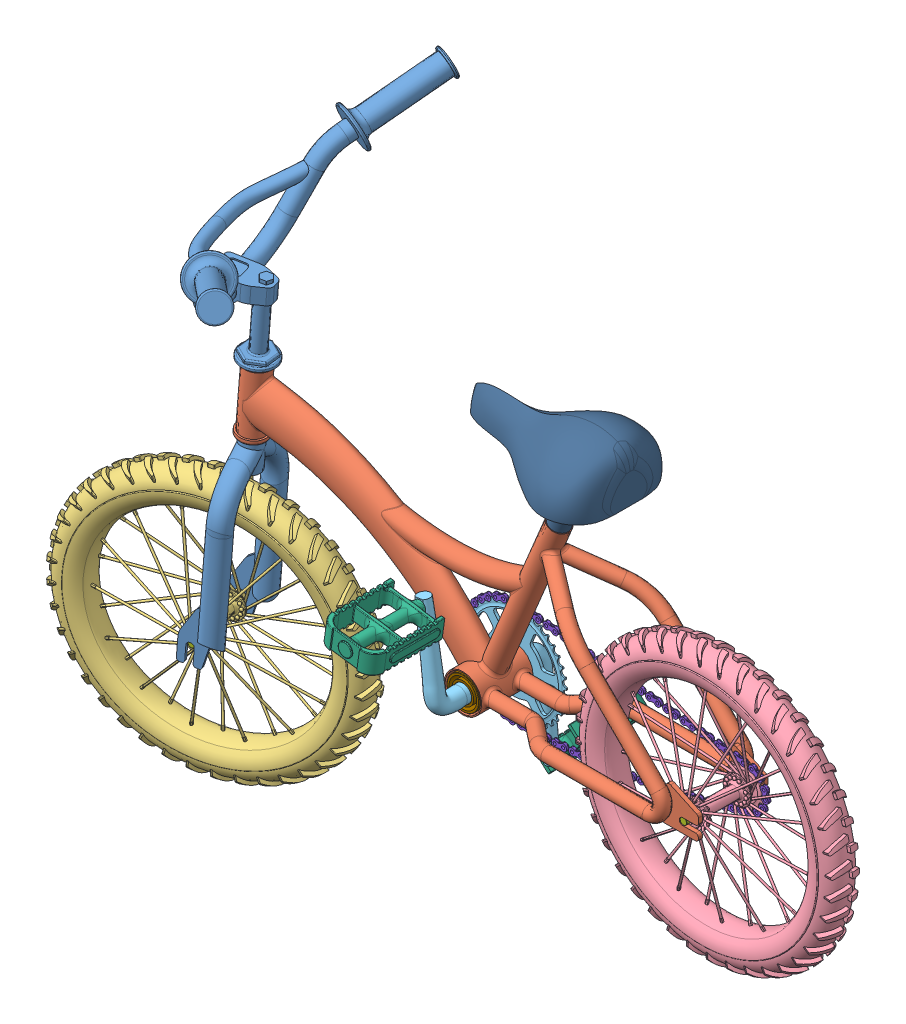
SolidWorks assembly Złożenierower, configuration Domyślna. Lengths in mm.
Overall size (1238.71 868.15 536.88).
12 component instances, 10 part files, 24 mates.
Components (placement in the parent):
- rower 1-1: rower 1 [Domyślna] at (-43.4947 150.1532 689.5871) x (0.960692 -0.078308 -0.266344) z (0.265464 -0.021639 0.963878) size (154.93 662.1 514.19)
- Część2-1: Część2 [Domyślna] at (307.1756 -163.303 684.2602) size (723.47 282.62 139.06)
- Część4-2: Część4 [Domyślna] at (-84.7109 -280.6724 691.2667) x (0.955551 -0.127096 -0.266024) z (0.265464 -0.021639 0.963878) size (399.15 399.28 100)
- Część3-1: Część3 [Domyślna] at (642.2913 -151.643 684.2602) x (0.731915 -0.681396 0) z (0 0 1) size (399.15 399.28 89)
- Część5-1: Część5 [Domyślna] at (307.1756 -163.303 685.2602) x (-0.14018 0.990126 0) z (0 0 1) size (270.08 150.67 176.37)
- Część9-1: Część9 [Domyślna] at (289.6531 -39.5372 827.2602) x (0 0 -1) z (0.990192 -0.139713 0) size (110.71 30.09 84)
- Część9-2: Część9 [Domyślna] at (324.6981 -287.0688 543.2602) x (0 0 1) z (0.66893 0.743326 0) size (110.71 30.09 84)
- Część8-1: Część8 [Domyślna] at (-84.7109 -280.6724 691.2667) x (0.911361 0.331819 -0.243551) z (0.265464 -0.021639 0.963878) size (10 10 100)
- Część8-2: Część8 [Domyślna] at (642.2913 -151.643 684.2602) x (1 -0.000733 0) z (0 0 1) size (10 10 100)
- Część7-2: Część7 [Domyślna] at (434.3029 -101.1447 643.7602) x (-0.994614 0.103648 0) z (0 0 -1) size (447.75 160.33 4)
- radial ball bearing_68_am-2: radial ball bearing_68_am [AFBMA 20.1 - 60-25 - 14,SI,NC,14_68] at (307.1756 -163.303 701.7602) x (0 0 -1) z (1 0 0) size (40 47 47)
- Część6-2: Część6 [Domyślna] at (397.1598 161.7409 684.2602) x (0.999017 -0.044322 0) z (0 0 1) size (231.81 225.72 159.65)
Mates (geometry in assembly coordinates):
- Koncentryczne1: concentric anti-aligned: cylinder of rower 1-1 through (-29.8866 79.8152 684.2602) axis (-0.081243 -0.996694 0) radius 15; cylinder of Część2-1 through (-51.9685 -191.087 684.2602) axis (0.081243 0.996694 0) radius 16
- Wspólnie2: coincident anti-aligned: plane of rower 1-1 through (-30.2928 74.8317 684.2602) normal (-0.081243 -0.996694 0); plane of Część2-1 through (-30.2928 74.8317 684.2602) normal (0.081243 0.996694 0)
- Koncentryczne3: concentric anti-aligned: cylinder of rower 1-1 through (-70.3758 -281.8409 743.3161) axis (-0.265464 0.021639 -0.963878) radius 5; cylinder of Część4-2 through (-94.9312 -279.8393 654.1574) axis (0.265464 -0.021639 0.963878) radius 5
- Szerokość1: width anti-aligned: plane of rower 1-1 through (-99.0459 -279.5039 639.2173) normal (-0.265464 0.021639 -0.963878); plane of Część4-2 through (-70.3758 -281.8409 743.3161) normal (0.265464 -0.021639 0.963878); plane of rower 1-1 through (-74.4905 -281.5055 728.376) normal (0.265464 -0.021639 0.963878); plane of Część4-2 through (-94.9312 -279.8393 654.1574) normal (-0.265464 0.021639 -0.963878)
- Koncentryczne4: concentric aligned: cylinder of Część2-1 through (642.2913 -151.643 729.2602) axis (0 0 1) radius 5; cylinder of Część3-1 through (642.2913 -151.643 645.7602) axis (0 0 1) radius 8.8
- Szerokość2: width aligned: plane of Część3-1 through (642.2913 -151.643 728.7602) normal (0 0 1); plane of Część2-1 through (642.2913 -151.643 639.7602) normal (0 0 -1); plane of Część3-1 through (622.4346 -118.5795 735.2602) normal (0 0 1); plane of Część2-1 through (622.4346 -118.5795 633.2602) normal (0 0 -1)
- Koncentryczne5: concentric anti-aligned: cylinder of Część2-1 through (307.1756 -163.303 614.7308) axis (0 0 1) radius 26; cylinder of Część5-1 through (307.1756 -163.303 727.7602) axis (0 0 -1) radius 12.5
- Wspólnie3: coincident anti-aligned: plane of Część2-1 through (307.1756 -163.303 646.7602) normal (0 0 -1); plane of Część5-1 through (269.7983 -168.5948 646.7602) normal (0 0 1)
- Koncentryczne6: concentric anti-aligned: cylinder of Część5-1 through (289.6531 -39.5372 535.2602) axis (0 0 1) radius 5; cylinder of Część9-1 through (289.6531 -39.5372 877.2602) axis (0 0 -1) radius 7.5
- Wspólnie4: coincident anti-aligned: plane of Część5-1 through (303.1032 -27.5333 767.2602) normal (0 0 1); plane of Część9-1 through (289.6531 -39.5372 767.2602) normal (0 0 -1)
- Koncentryczne7: concentric aligned: cylinder of Część5-1 through (324.6981 -287.0688 535.2602) axis (0 0 1) radius 5; cylinder of Część9-2 through (324.6981 -287.0688 493.2602) axis (0 0 1) radius 7.5
- Wspólnie5: coincident anti-aligned: plane of Część5-1 through (340.9517 -294.8673 603.2602) normal (0 0 -1); plane of Część9-2 through (324.6981 -287.0688 603.2602) normal (0 0 1)
- Koncentryczne8: concentric aligned: cylinder of Część4-2 through (-72.8977 -281.6353 734.1593) axis (-0.265464 0.021639 -0.963878) radius 5; cylinder of Część8-1 through (-71.4377 -281.7543 739.4606) axis (-0.265464 0.021639 -0.963878) radius 5
- Szerokość3: width anti-aligned: plane of Część8-1 through (-71.4377 -281.7543 739.4606) normal (0.265464 -0.021639 0.963878); plane of rower 1-1 through (-97.9841 -279.5905 643.0728) normal (-0.265464 0.021639 -0.963878); plane of Część8-1 through (-71.4377 -281.7543 739.4606) normal (-0.265464 0.021639 -0.963878); plane of rower 1-1 through (-97.9841 -279.5905 643.0728) normal (0.265464 -0.021639 0.963878)
- Koncentryczne9: concentric anti-aligned: cylinder of Część3-1 through (642.2913 -151.643 645.7602) axis (0 0 1) radius 5; cylinder of Część8-2 through (642.2913 -151.643 734.2602) axis (0 0 -1) radius 5
- Szerokość4: width anti-aligned: plane of Część8-2 through (642.2913 -151.643 734.2602) normal (0 0 1); plane of Część2-1 through (642.2913 -151.643 634.2602) normal (0 0 -1); plane of Część8-2 through (622.4346 -118.5795 729.2602) normal (0 0 -1); plane of Część2-1 through (622.4346 -118.5795 639.2602) normal (0 0 1)
- Koncentryczne12: concentric anti-aligned: circle of Część5-1; circle of Część7-2
- Wspólnie8: coincident aligned: plane of Część3-1 through (662.1131 -130.3516 641.7602) normal (0 0 -1); plane of Część7-2 through (677.2831 -144.2992 641.7602) normal (0 0 -1)
- Zablokuj2: lock: unknown of Część3-1; unknown of Część7-2
- Koncentryczne13: concentric aligned: cylinder of Część5-1 through (307.1756 -163.303 727.7602) axis (0 0 -1) radius 12.5; cylinder of radial ball bearing_68_am-2 through (307.1756 -163.303 722.3977) axis (0 0 -1) radius 12.5
- Wspólnie11: coincident aligned: plane of Część2-1 through (307.1756 -163.303 721.7602) normal (0 0 1); plane of radial ball bearing_68_am-2 through (307.1756 -143.103 721.7602) normal (0 0 1)
- Koncentryczne14: concentric: cylinder of Część2-1 through (244.1524 -315.1521 684.2602) axis (0.383333 0.92361 0) radius 13.5; cylinder of Część6-2 through (383.8423 21.419 684.2602) axis (0.383333 0.92361 0) radius 14
- Odległość2: distance = 90 mm: plane of Część6-2 through (417.0276 180.8791 649.2602) normal (-0.383333 -0.92361 0); plane of Część2-1 through (410.6756 86.0717 684.2602) normal (0.383333 0.92361 0)
- Wspólnie14: coincident aligned: plane of Część2-1 through (307.1756 -163.303 684.2602) normal (0 0 1); plane of Część6-2 through (397.1598 161.7409 684.2602) normal (0 0 1)
